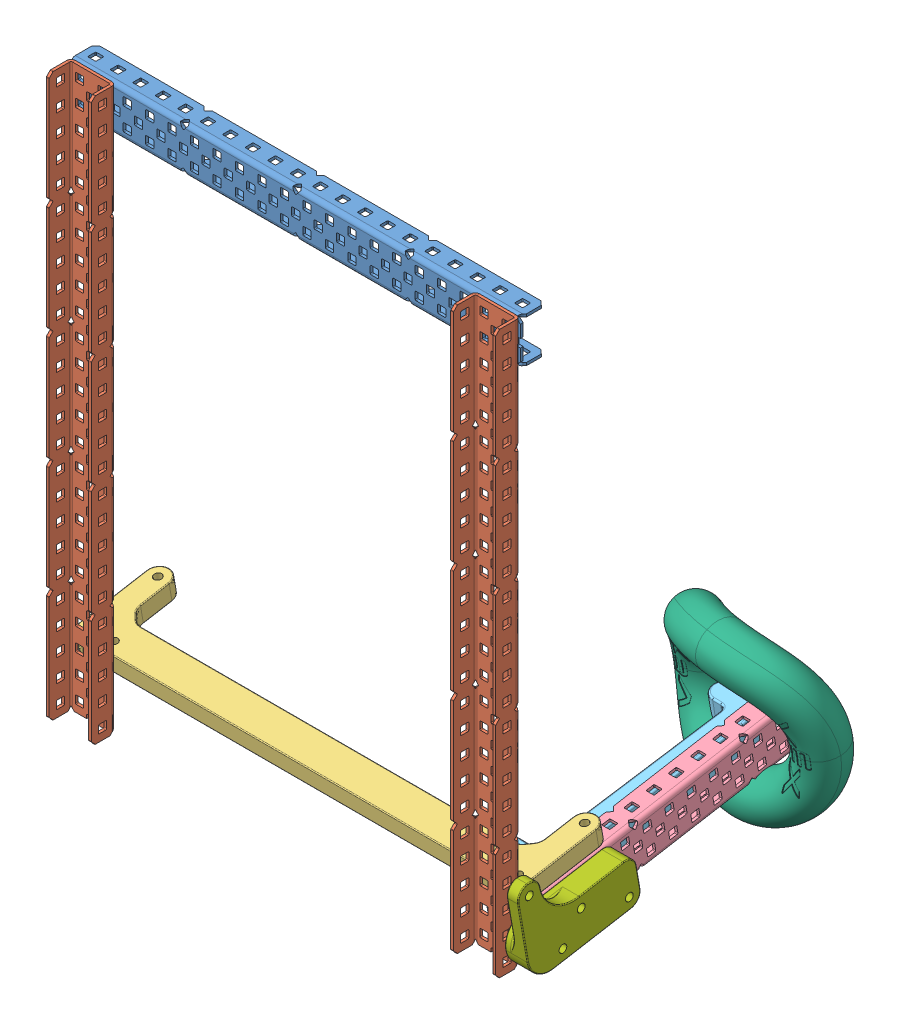
SolidWorks assembly TestFit, configuration Default. Lengths in mm.
Overall size (295.5 344.52 196.4).
13 component instances, 7 part files, 8 mates.
Components (placement in the parent):
- 1x2x1x20 Aluminum C-Channel-1: 1x2x1x20 Aluminum C-Channel [Default] at (209.9542 137.9284 187.8001) size (254 25.41 13.97)
- 1x2x1x25 Aluminum C-Channel (276-2289)-1: 1x2x1x25 Aluminum C-Channel (276-2289) [Default] at (229.0042 -71.6216 187.8001) x (0 -1 0) z (0 0 -1) size (317.5 25.41 13.97)
- 1x2x1x25 Aluminum C-Channel (276-2289)-2: 1x2x1x25 Aluminum C-Channel (276-2289) [Default] at (0.4042 -71.6216 187.8001) x (0 -1 0) z (0 0 -1) size (317.5 25.41 13.97)
- RingMechAssem-1: RingMechAssem [Default] at (251.768 -296.6408 336.1194) x (-1 0 0) z (0 0.169666 -0.985502) size (295.5 104.58 181.29)
  - top_brace-1: top_brace [Default] at (138.3338 128.7715 174.5683) size (254 10 50.8)
  - 1x2x1x12 Aluminum C-Channel-1: 1x2x1x12 Aluminum C-Channel [Default] at (10.0638 116.0715 396.8183) x (0 0 1) z (-1 0 0) size (152.4 25.41 13.97)
  - ring_hook-1: ring_hook [Default] at (24.1322 103.3715 174.4714) x (0.999882 0 0.015379) z (-0.015379 0 0.999882) size (38.1 19.4 152.4)
  - Ring-1: Ring [Default] at (50.2974 128.7715 319.8409) x (0.992006 0 0.126195) z (0 1 0) size (101.61 43.55 104.58)
    - Ring.step-1: Ring.step [Default] at origin size (101.61 43.55 104.58)
      - 276-7048-350 Rev2.step-1: 276-7048-350 Rev2.step [Default] at (-27.7593 -20.073 1639.1281) size (101.61 43.55 104.58)
        - 276-7048-301 Rev2 (1).step-1: 276-7048-301 Rev2 (1).step [Default] at (0 0 -1197.0106) x (0 0 -1) z (1 0 0) size (104.58 43.55 101.61)
          - 276-7048-001 Rev2.step-1: 276-7048-001 Rev2.step [Default] at (442.1175 9.4315 0) size (104.58 43.55 101.61)
  - hinge-1: hinge [Default] at (3.7138 154.1715 161.8683) x (0 0 1) z (0 -1 0) size (63.99 12.7 50.8)
Mates (geometry in assembly coordinates):
- Coincident8: coincident anti-aligned: plane of 1x2x1x20 Aluminum C-Channel-1 through (-11.7958 116.0081 187.8001) normal (0 0 1); plane of 1x2x1x25 Aluminum C-Channel (276-2289)-1 through (250.9245 150.1284 187.8001) normal (0 0 -1)
- Coincident9: coincident anti-aligned: plane of 1x2x1x20 Aluminum C-Channel-1 through (-11.7958 116.0081 187.8001) normal (0 0 1); plane of 1x2x1x25 Aluminum C-Channel (276-2289)-2 through (22.3245 150.1284 187.8001) normal (0 0 -1)
- Coincident10: coincident aligned: plane of 1x2x1x20 Aluminum C-Channel-1 through (-11.7958 150.6284 220.1588) normal (0 1 0); plane of 1x2x1x25 Aluminum C-Channel (276-2289)-2 through (22.3245 150.6284 189.3749) normal (0 1 0)
- Coincident11: coincident anti-aligned: circle of 1x2x1x20 Aluminum C-Channel-1; circle of 1x2x1x25 Aluminum C-Channel (276-2289)-2
- Coincident12: coincident aligned: plane of 1x2x1x20 Aluminum C-Channel-1 through (-11.7958 150.6284 220.1588) normal (0 1 0); plane of 1x2x1x25 Aluminum C-Channel (276-2289)-1 through (250.9245 150.6284 189.3749) normal (0 1 0)
- Coincident13: coincident anti-aligned: circle of 1x2x1x20 Aluminum C-Channel-1; circle of 1x2x1x25 Aluminum C-Channel (276-2289)-1
- Concentric1: concentric anti-aligned: circle of 1x2x1x25 Aluminum C-Channel (276-2289)-1; circle of RingMechAssem-1/hinge-1
- Coincident14: coincident anti-aligned: plane of 1x2x1x25 Aluminum C-Channel (276-2289)-1 through (241.7042 150.1284 199.282) normal (1 0 0); plane of RingMechAssem-1/hinge-1 through (241.7042 -117.2411 202.7554) normal (-1 0 0)
